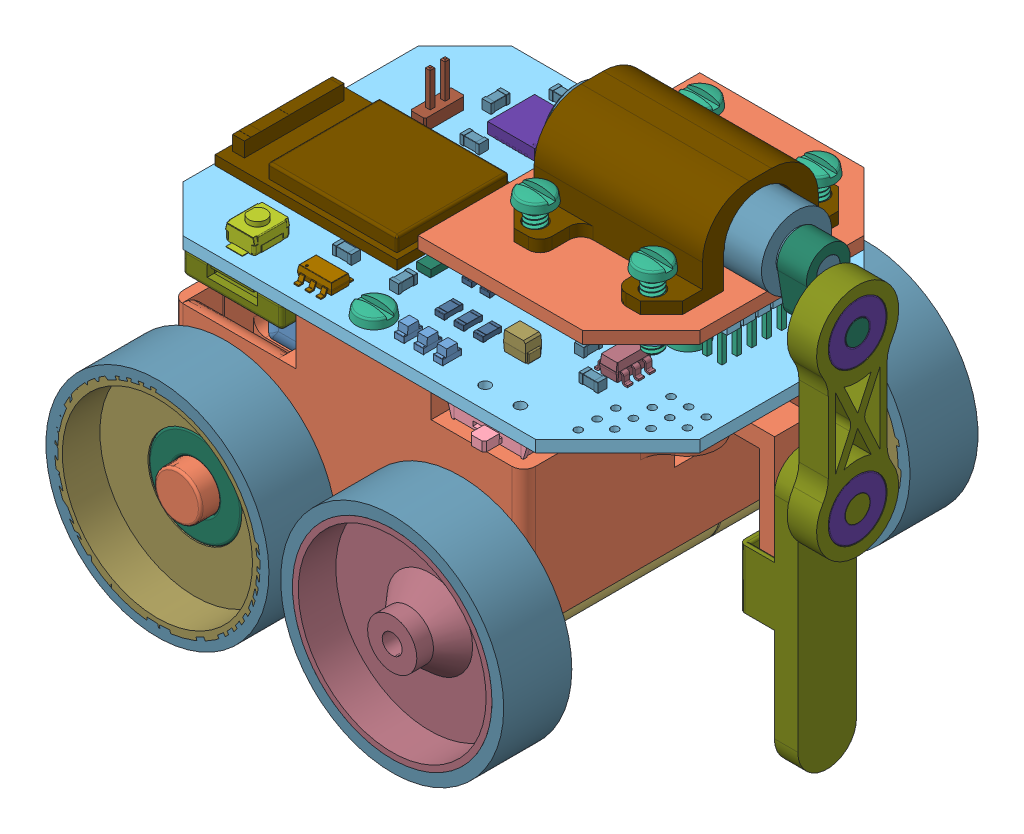
SolidWorks assembly AstroAnt_knock, configuration Default. Lengths in mm.
Overall size (52.98 43.52 40.4).
186 component instances, 53 part files, 54 mates.
Components (placement in the parent):
- LiPo_360mAh-1: LiPo_360mAh [Default] at (6.8166 4.9998 44.2756) size (25 7 18)
- Body-1: Body [Default] at (4.8007 -0.0002 38.7677) size (39 16 37)
- PA2-50-1: PA2-50 [Default] at (8.0673 -18.301 41.8029) x (0 0 1) z (0.952879 0.303349 0) size (29.1 8 8)
- PA2-50-2: PA2-50 [Default] at (-4.1563 19.5334 49.6029) x (0 0 -1) z (0.755989 -0.654584 0) size (29.1 8 8)
- 92120A150_Brass Heat-Set Inserts for Plastic-1: 92120A150_Brass Heat-Set Inserts for Plastic [92120A150] at (19.9543 12.4998 45.7029) size (2.56 3.33 2.56)
- 92120A150_Brass Heat-Set Inserts for Plastic-2: 92120A150_Brass Heat-Set Inserts for Plastic [92120A150] at (4.9543 12.4998 33.9529) size (2.56 3.33 2.56)
- 92120A150_Brass Heat-Set Inserts for Plastic-3: 92120A150_Brass Heat-Set Inserts for Plastic [92120A150] at (4.9543 12.4998 57.4529) size (2.56 3.33 2.56)
- motor_holder-1: motor_holder [Default] at (-0.192 -4.5002 11.9282) size (20 4.13 28)
- 91460A005_METRIC CHEESE HEAD SLOTTED MACHINE SCREW-8: 91460A005_METRIC CHEESE HEAD SLOTTED MACHINE SCREW [91460A005] at (4.9543 14.9998 57.4529) x (1 0 0) z (0 1 0) size (3 3 7.1)
- 91460A005_METRIC CHEESE HEAD SLOTTED MACHINE SCREW-9: 91460A005_METRIC CHEESE HEAD SLOTTED MACHINE SCREW [91460A005] at (4.9543 14.9998 33.9529) x (1 0 0) z (0 1 0) size (3 3 7.1)
- 91460A005_METRIC CHEESE HEAD SLOTTED MACHINE SCREW-10: 91460A005_METRIC CHEESE HEAD SLOTTED MACHINE SCREW [91460A005] at (19.9543 14.9998 45.7029) x (1 0 0) z (0 1 0) size (3 3 7.1)
- 92120A150_Brass Heat-Set Inserts for Plastic-4: 92120A150_Brass Heat-Set Inserts for Plastic [92120A150] at (4.9543 1.4998 57.4529) x (-0.616962 0 -0.786993) z (0.786993 0 -0.616962) size (2.56 3.33 2.56)
- 92120A150_Brass Heat-Set Inserts for Plastic-5: 92120A150_Brass Heat-Set Inserts for Plastic [92120A150] at (4.9543 1.4998 33.9529) x (-0.616962 0 -0.786993) z (0.786993 0 -0.616962) size (2.56 3.33 2.56)
- 91460A005_METRIC CHEESE HEAD SLOTTED MACHINE SCREW-14: 91460A005_METRIC CHEESE HEAD SLOTTED MACHINE SCREW [91460A005] at (4.9543 -2.5002 57.4529) x (0.663599 0 0.748089) z (0 -1 0) size (3 3 7.1)
- 91460A005_METRIC CHEESE HEAD SLOTTED MACHINE SCREW-15: 91460A005_METRIC CHEESE HEAD SLOTTED MACHINE SCREW [91460A005] at (4.9543 -2.5002 33.9529) x (0.663599 0 0.748089) z (0 -1 0) size (3 3 7.1)
- mainboard_v1.step-1: mainboard_v1.step [Default] at (-103.0457 13.9998 235.7029) x (0 0 -1) z (0 1 0) size (29.41 41 10.8)
  - B3U-1000P.step-1: B3U-1000P.step [Default] at (178.95 -97.38 1.05) x (1 0 0) z (0 -1 0) size (4 1.75 2.5)
    - COMPOUND.step-1: COMPOUND.step [Default] at origin size (4 1.75 2.5)
  - 20021321-00014C1LF.step-1: 20021321-00014C1LF.step [Default] at (190 -115.5 1.05) size (9.35 5.45 4.85)
    - COMPOUND-0.step-1: COMPOUND-0.step [Default] at origin size (9.35 5.45 4.85)
  - MP6513GJ-Z.step-1: MP6513GJ-Z.step [Default] at (201.21 -120 1.05) x (-1 0 0) z (0 0 1) size (2.8 2.9 1)
    - COMPOUND-1.step-1: COMPOUND-1.step [Default] at origin size (2.8 2.9 1)
  - MP6513GJ-Z.step-2: MP6513GJ-Z.step [Default] at (178.51 -103.46 1.05) size (2.8 2.9 1)
    - COMPOUND-1.step-1: COMPOUND-1.step [Default] at origin size (2.8 2.9 1)
  - R_0603_1608Metric.step-1: R_0603_1608Metric.step [Default] at (195.55 -104.38 -0.05) x (1 0 0) z (0 0 -1) size (1.6 0.8 0.45)
    - SOLID.step-1: SOLID.step [Default] at origin size (1.6 0.8 0.45)
  - R_0603_1608Metric.step-2: R_0603_1608Metric.step [Default] at (192.6 -99.86 -0.05) x (0 1 0) z (0 0 -1) size (1.6 0.8 0.45)
    - SOLID.step-1: SOLID.step [Default] at origin size (1.6 0.8 0.45)
  - PinHeader_2x01_P1.27mm_Vertical.step-1: PinHeader_2x01_P1.27mm_Vertical.step [Default] at (194.96 -96.07 1.05) size (3.4 1.27 6.3)
    - SOLID-2.step-1: SOLID-2.step [Default] at origin size (3.4 1.27 6.3)
  - TAJP106K010RNJ.step-1: TAJP106K010RNJ.step [Default] at (196.22 -98.14 -0.05) x (-1 0 0) z (0 0 -1) size (2.05 1.4 1.7)
    - COMPOUND-3.step-1: COMPOUND-3.step [Default] at origin size (2.05 1.4 1.7)
  - TAJP106K010RNJ.step-2: TAJP106K010RNJ.step [Default] at (181.68 -117.23 1.05) x (0 1 0) z (0 0 1) size (2.05 1.4 1.7)
    - COMPOUND-3.step-1: COMPOUND-3.step [Default] at origin size (2.05 1.4 1.7)
  - SOT-23-5.step-1: SOT-23-5.step [Default] at (195.38 -122.78 1.05) x (0 1 0) z (0 0 1) size (2.8 2.9 1.55)
    - SOLID-4.step-1: SOLID-4.step [Default] at origin size (2.8 2.9 1.55)
  - C_0603_1608Metric.step-1: C_0603_1608Metric.step [Default] at (192.91 -122.55 1.05) x (0 -1 0) z (0 0 1) size (1.6 0.8 0.8)
    - SOLID-5.step-1: SOLID-5.step [Default] at origin size (1.6 0.8 0.8)
  - C_0603_1608Metric.step-2: C_0603_1608Metric.step [Default] at (193.57 -119.76 1.05) size (1.6 0.8 0.8)
    - SOLID-5.step-1: SOLID-5.step [Default] at origin size (1.6 0.8 0.8)
  - ECS-.327-12.5-12-TR.step-1: ECS-.327-12.5-12-TR.step [Default] at (184.31 -107.18 1.05) size (2 1.2 0.7)
    - COMPOUND-6.step-1: COMPOUND-6.step [Default] at origin size (2 1.2 0.7)
  - C_0603_1608Metric.step-3: C_0603_1608Metric.step [Default] at (197.67 -113.69 1.05) size (1.6 0.8 0.8)
    - SOLID-5.step-1: SOLID-5.step [Default] at origin size (1.6 0.8 0.8)
  - C_0603_1608Metric.step-4: C_0603_1608Metric.step [Default] at (197.64 -107.18 1.05) size (1.6 0.8 0.8)
    - SOLID-5.step-1: SOLID-5.step [Default] at origin size (1.6 0.8 0.8)
  - C_0603_1608Metric.step-5: C_0603_1608Metric.step [Default] at (190.96 -108.09 1.05) x (0 1 0) z (0 0 1) size (1.6 0.8 0.8)
    - SOLID-5.step-1: SOLID-5.step [Default] at origin size (1.6 0.8 0.8)
  - 1734592-6.step-1: 1734592-6.step [Default] at (203.79 -118 -1.05) x (0 -1 0) z (1 0 0) size (8.43 2.05 5.11)
    - SOLID-7.step-1: SOLID-7.step [Default] at origin size (8.43 2.05 5.11)
  - 1734592-6.step-2: 1734592-6.step [Default] at (176.19 -98 -1.05) x (0 1 0) z (-1 0 0) size (8.43 2.05 5.11)
    - SOLID-7.step-1: SOLID-7.step [Default] at origin size (8.43 2.05 5.11)
  - 20021321-00010C4LF.step-1: 20021321-00010C4LF.step [Default] at (190 -127.85 -0.05) x (1 0 0) z (0 0 -1) size (6.81 5.45 4.85)
    - COMPOUND-8.step-1: COMPOUND-8.step [Default] at origin size (6.81 5.45 4.85) (hidden)
  - 20021321-00010C4LF.step-2: 20021321-00010C4LF.step [Default] at (190 -127.85 1.05) size (6.81 5.45 4.85)
    - COMPOUND-8.step-1: COMPOUND-8.step [Default] at origin size (6.81 5.45 4.85) (hidden)
  - C_0603_1608Metric.step-6: C_0603_1608Metric.step [Default] at (181.31 -102.6 1.05) x (0 -1 0) z (0 0 1) size (1.6 0.8 0.8)
    - SOLID-5.step-1: SOLID-5.step [Default] at origin size (1.6 0.8 0.8)
  - C_0603_1608Metric.step-7: C_0603_1608Metric.step [Default] at (198.25 -119.14 1.05) x (0 -1 0) z (0 0 1) size (1.6 0.8 0.8)
    - SOLID-5.step-1: SOLID-5.step [Default] at origin size (1.6 0.8 0.8)
  - MPU6050.step-1: MPU6050.step [Default] at (198.43 -101.5 1.05) x (0 1 0) z (1 0 0) size (4 0.95 4)
    - COMPOUND-9.step-1: COMPOUND-9.step [Default] at origin size (4 0.95 4)
  - C_0603_1608Metric.step-8: C_0603_1608Metric.step [Default] at (194.9 -99.89 1.05) x (0 -1 0) z (0 0 1) size (1.6 0.8 0.8)
    - SOLID-5.step-1: SOLID-5.step [Default] at origin size (1.6 0.8 0.8)
  - C_0603_1608Metric.step-9: C_0603_1608Metric.step [Default] at (201.98 -100.38 1.05) x (0 -1 0) z (0 0 1) size (1.6 0.8 0.8)
    - SOLID-5.step-1: SOLID-5.step [Default] at origin size (1.6 0.8 0.8)
  - C_0603_1608Metric.step-10: C_0603_1608Metric.step [Default] at (201.98 -103.78 1.05) x (0 1 0) z (0 0 1) size (1.6 0.8 0.8)
    - SOLID-5.step-1: SOLID-5.step [Default] at origin size (1.6 0.8 0.8)
  - C_0603_1608Metric.step-11: C_0603_1608Metric.step [Default] at (198.81 -97.82 1.05) size (1.6 0.8 0.8)
    - SOLID-5.step-1: SOLID-5.step [Default] at origin size (1.6 0.8 0.8)
  - SOT-23-5.step-2: SOT-23-5.step [Default] at (184.86 -122.77 1.05) x (0 1 0) z (0 0 1) size (2.8 2.9 1.55)
    - SOLID-4.step-1: SOLID-4.step [Default] at origin size (2.8 2.9 1.55)
  - SOT-23-5.step-3: SOT-23-5.step [Default] at (197.58 -110.46 1.05) x (0 1 0) z (0 0 1) size (2.8 2.9 1.55)
    - SOLID-4.step-1: SOLID-4.step [Default] at origin size (2.8 2.9 1.55)
  - MDBT50Q-1MV2.step-1: MDBT50Q-1MV2.step [Default] at (187.3136 -98.605 1.0754) x (-1 0 0) z (0 1 0) size (10.5 2.06 15.5)
    - SOLID-10.step-1: SOLID-10.step [Default] at origin size (10.5 2.06 15.5)
  - C_0603_1608Metric.step-12: C_0603_1608Metric.step [Default] at (189.44 -108.09 1.05) x (0 1 0) z (0 0 1) size (1.6 0.8 0.8)
    - SOLID-5.step-1: SOLID-5.step [Default] at origin size (1.6 0.8 0.8)
  - C_0603_1608Metric.step-13: C_0603_1608Metric.step [Default] at (181.57 -107.18 1.05) x (-1 0 0) z (0 0 1) size (1.6 0.8 0.8)
    - SOLID-5.step-1: SOLID-5.step [Default] at origin size (1.6 0.8 0.8)
  - C_0603_1608Metric.step-14: C_0603_1608Metric.step [Default] at (186.97 -107.18 1.05) size (1.6 0.8 0.8)
    - SOLID-5.step-1: SOLID-5.step [Default] at origin size (1.6 0.8 0.8)
  - C_0603_1608Metric.step-15: C_0603_1608Metric.step [Default] at (184.77 -119.75 1.05) x (-1 0 0) z (0 0 1) size (1.6 0.8 0.8)
    - SOLID-5.step-1: SOLID-5.step [Default] at origin size (1.6 0.8 0.8)
  - C_0603_1608Metric.step-16: C_0603_1608Metric.step [Default] at (182.37 -122.54 1.05) x (0 -1 0) z (0 0 1) size (1.6 0.8 0.8)
    - SOLID-5.step-1: SOLID-5.step [Default] at origin size (1.6 0.8 0.8)
  - LED_0603_1608Metric.step-1: LED_0603_1608Metric.step [Default] at (178.19 -111.01 1.05) size (1.6 0.8 1.1)
    - SOLID-11.step-1: SOLID-11.step [Default] at origin size (1.6 0.8 1.1)
  - LED_0603_1608Metric.step-2: LED_0603_1608Metric.step [Default] at (178.19 -112.66 1.05) size (1.6 0.8 1.1)
    - SOLID-11.step-1: SOLID-11.step [Default] at origin size (1.6 0.8 1.1)
  - LED_0603_1608Metric.step-3: LED_0603_1608Metric.step [Default] at (178.19 -114.31 1.05) size (1.6 0.8 1.1)
    - SOLID-11.step-1: SOLID-11.step [Default] at origin size (1.6 0.8 1.1)
  - LED_0603_1608Metric.step-4: LED_0603_1608Metric.step [Default] at (202.34 -112.21 1.05) x (0 1 0) z (0 0 1) size (1.6 0.8 1.1)
    - SOLID-11.step-1: SOLID-11.step [Default] at origin size (1.6 0.8 1.1)
  - 473460001.step-1: 473460001.step [Default] at (201.68 -99.72 -1.25) x (0 -1 0) z (1 0 0) size (7.98 2.94 5.43)
    - COMPOUND-12.step-1: COMPOUND-12.step [Default] at origin size (7.98 2.94 5.43)
  - L_0603_1608Metric.step-1: L_0603_1608Metric.step [Default] at (192.48 -108.09 1.05) x (0 1 0) z (0 0 1) size (1.6 0.8 0.8)
    - SOLID-13.step-1: SOLID-13.step [Default] at origin size (1.6 0.8 0.8)
  - R_0603_1608Metric.step-3: R_0603_1608Metric.step [Default] at (185.18 -111.31 1.05) x (-1 0 0) z (0 0 1) size (1.6 0.8 0.45)
    - SOLID.step-1: SOLID.step [Default] at origin size (1.6 0.8 0.45)
  - R_0603_1608Metric.step-4: R_0603_1608Metric.step [Default] at (185.18 -109.77 1.05) size (1.6 0.8 0.45)
    - SOLID.step-1: SOLID.step [Default] at origin size (1.6 0.8 0.45)
  - R_0603_1608Metric.step-5: R_0603_1608Metric.step [Default] at (181.62 -111.01 1.05) size (1.6 0.8 0.45)
    - SOLID.step-1: SOLID.step [Default] at origin size (1.6 0.8 0.45)
  - R_0603_1608Metric.step-6: R_0603_1608Metric.step [Default] at (181.62 -112.66 1.05) size (1.6 0.8 0.45)
    - SOLID.step-1: SOLID.step [Default] at origin size (1.6 0.8 0.45)
  - R_0603_1608Metric.step-7: R_0603_1608Metric.step [Default] at (181.62 -114.31 1.05) x (-1 0 0) z (0 0 1) size (1.6 0.8 0.45)
    - SOLID.step-1: SOLID.step [Default] at origin size (1.6 0.8 0.45)
  - R_0603_1608Metric.step-8: R_0603_1608Metric.step [Default] at (194.84 -108.1 1.05) x (0 1 0) z (0 0 1) size (1.6 0.8 0.45)
    - SOLID.step-1: SOLID.step [Default] at origin size (1.6 0.8 0.45)
  - R_0603_1608Metric.step-9: R_0603_1608Metric.step [Default] at (200.69 -112.2325 1.05) x (0 1 0) z (0 0 1) size (1.6 0.8 0.45)
    - SOLID.step-1: SOLID.step [Default] at origin size (1.6 0.8 0.45)
  - R_0603_1608Metric.step-10: R_0603_1608Metric.step [Default] at (196.22 -101.51 -0.05) x (-1 0 0) z (0 0 -1) size (1.6 0.8 0.45)
    - SOLID.step-1: SOLID.step [Default] at origin size (1.6 0.8 0.45)
  - R_0603_1608Metric.step-11: R_0603_1608Metric.step [Default] at (196.22 -99.9725 -0.05) x (-1 0 0) z (0 0 -1) size (1.6 0.8 0.45)
    - SOLID.step-1: SOLID.step [Default] at origin size (1.6 0.8 0.45)
  - SW_SPDT_PCM12.step-1: SW_SPDT_PCM12.step [Default] at (178.18 -119.37 -0.05) x (0 1 0) z (0 0 -1) size (7.7 5 2)
    - SOLID-14.step-1: SOLID-14.step [Default] at origin size (7.7 5 2)
  - COMPOUND-15.step-1: COMPOUND-15.step [Default] at origin size (28 41 1)
- 91613A020_METRIC CHEESE HEAD SLOTTED MACHINE SCREW-1: 91613A020_METRIC CHEESE HEAD SLOTTED MACHINE SCREW [91613A020] at (1.2533 -0.5002 54.4029) x (1 0 0) z (0 1 0) size (3 3 5.08)
- 91613A020_METRIC CHEESE HEAD SLOTTED MACHINE SCREW-2: 91613A020_METRIC CHEESE HEAD SLOTTED MACHINE SCREW [91613A020] at (8.6533 -0.5002 54.4029) x (1 0 0) z (0 1 0) size (3 3 5.08)
- 91613A020_METRIC CHEESE HEAD SLOTTED MACHINE SCREW-3: 91613A020_METRIC CHEESE HEAD SLOTTED MACHINE SCREW [91613A020] at (1.2533 -0.5002 37.0029) x (1 0 0) z (0 1 0) size (3 3 5.08)
- IR_TEMP_V2.step-3: IR_TEMP_V2.step [Default] at (118.9553 -0.5002 109.7029) x (-1 0 0) z (0 1 0) size (10 20 4.8)
  - Board_Geoms_380f.step-1: Board_Geoms_380f.step [Default] at origin size (10 20 1.11)
    - Pcb_380f.step-1: Pcb_380f.step [Default] at origin size (10 20 1)
    - topTracks_380f.step-1: topTracks_380f.step [Default] at (0 0 0.01) size (9.62 17.53 0.05)
    - botTracks_380f.step-1: botTracks_380f.step [Default] at (0 0 -1.01) size (9.25 16.88 0.05)
  - Step_Models_380f.step-1: Step_Models_380f.step [Default] at origin size (9.46 10.17 4.8)
    - Top_380f.step-1: Top_380f.step [Default] at origin size (9.46 10.17 1.2)
      - IC1_PW14_613E6C6D.step-1: IC1_PW14_613E6C6D.step [Default] at (113.99 -59.48 0) x (-1 0 0) z (0 1 0) size (6.4 1.2 5)
      - C1_C_0402_1005Metric_613EDDF6.step-1: C1_C_0402_1005Metric_613EDDF6.step [Default] at (110.5 -64.26 0) x (-1 0 0) z (0 0 1) size (1 0.5 0.5)
      - C1_C_0402_1005Metric_613EDDF6.step-2: C1_C_0402_1005Metric_613EDDF6.step [Default] at (109.52 -61.07 0) x (0 -1 0) z (0 0 1) size (1 0.5 0.5)
      - C1_C_0402_1005Metric_613EDDF6.step-3: C1_C_0402_1005Metric_613EDDF6.step [Default] at (118.48 -60.86 0) x (0 -1 0) z (0 0 1) size (1 0.5 0.5)
      - C1_C_0402_1005Metric_613EDDF6.step-4: C1_C_0402_1005Metric_613EDDF6.step [Default] at (118.48 -58.59 0) x (0 -1 0) z (0 0 1) size (1 0.5 0.5)
      - C1_C_0402_1005Metric_613EDDF6.step-5: C1_C_0402_1005Metric_613EDDF6.step [Default] at (113.32 -66.9 0) size (1 0.5 0.5)
      - R1_R_0402_1005Metric_613EDE7A.step-1: R1_R_0402_1005Metric_613EDE7A.step [Default] at (110.98 -63.1 0) size (1 0.5 0.35)
      - R1_R_0402_1005Metric_613EDE7A.step-2: R1_R_0402_1005Metric_613EDE7A.step [Default] at (111.68 -66.3 0) x (0 1 0) z (0 0 1) size (1 0.5 0.35)
    - Bot_380f.step-1: Bot_380f.step [Default] at origin size (6.35 7.64 4.6)
      - U1_ZTP-135SR_613E6CD4.step-1: U1_ZTP-135SR_613E6CD4.step [Default] at (114 -64 -1) x (-1 0 0) z (0 -1 0) size (6.35 4.6 5.4)
      - C1_C_0402_1005Metric_613EDDF6.step-1: C1_C_0402_1005Metric_613EDDF6.step [Default] at (115.07 -59.56 -1) x (0 -1 0) z (0 0 -1) size (1 0.5 0.5)
      - R1_R_0402_1005Metric_613EDE7A.step-1: R1_R_0402_1005Metric_613EDE7A.step [Default] at (113.64 -59.58 -1) x (0 -1 0) z (0 0 -1) size (1 0.5 0.35)
- TGPP06-D-136-1: TGPP06-D-136 [Default] at (10.3043 25.9998 45.7013) x (0 0.096627 0.995321) z (1 0 0) size (6 6 21.6)
- knock_wheel-1: knock_wheel [Default] at (29.4043 58.5713 96.4623) x (1 0 0) z (0 -0.096627 -0.995321) size (5.3 6.04 3.72)
- knock_connect_bar-1: knock_connect_bar [Default] at (32.2043 -15.7821 12.5082) size (2.5 20 7)
- ball_bearing-1: ball_bearing [Default] at (32.2043 22.8882 46.0034) x (1 0 0) z (0 -0.605691 0.7957) size (2.5 5 5)
- ball_bearing-2: ball_bearing [Default] at (32.2043 9.8882 46.0034) size (2.5 5 5)
- knock_motor_holder-1: knock_motor_holder [Default] at (-0.3495 23.0998 0.3235) size (14.34 7 16.88)
- 91460A005_METRIC CHEESE HEAD SLOTTED MACHINE SCREW-16: 91460A005_METRIC CHEESE HEAD SLOTTED MACHINE SCREW [91460A005] at (23.9543 25.5998 38.7029) x (1 0 0) z (0 1 0) size (3 3 7.1)
- 91460A005_METRIC CHEESE HEAD SLOTTED MACHINE SCREW-17: 91460A005_METRIC CHEESE HEAD SLOTTED MACHINE SCREW [91460A005] at (13.9543 25.5998 38.7029) x (1 0 0) z (0 1 0) size (3 3 7.1)
- 91460A005_METRIC CHEESE HEAD SLOTTED MACHINE SCREW-18: 91460A005_METRIC CHEESE HEAD SLOTTED MACHINE SCREW [91460A005] at (23.9543 25.5998 52.7013) x (1 0 0) z (0 1 0) size (3 3 7.1)
- 91460A005_METRIC CHEESE HEAD SLOTTED MACHINE SCREW-19: 91460A005_METRIC CHEESE HEAD SLOTTED MACHINE SCREW [91460A005] at (13.9543 25.5998 52.7013) x (1 0 0) z (0 1 0) size (3 3 7.1)
- 90710A145_18-8 Stainless Steel Thin Hex Nut-1: 90710A145_18-8 Stainless Steel Thin Hex Nut [90710A145] at (23.9543 21.4998 52.7029) size (3.2 1.33 3.7)
- 90710A145_18-8 Stainless Steel Thin Hex Nut-2: 90710A145_18-8 Stainless Steel Thin Hex Nut [90710A145] at (23.9543 21.4998 38.7029) size (3.2 1.33 3.7)
- 90710A145_18-8 Stainless Steel Thin Hex Nut-3: 90710A145_18-8 Stainless Steel Thin Hex Nut [90710A145] at (13.9543 21.4998 38.7029) size (3.2 1.33 3.7)
- 90710A145_18-8 Stainless Steel Thin Hex Nut-4: 90710A145_18-8 Stainless Steel Thin Hex Nut [90710A145] at (13.9543 21.4998 52.7029) size (3.2 1.33 3.7)
- knock_driver.step-1: knock_driver.step [Default] at (27.9543 23.0401 52.7029) x (0 0 -1) z (0 1 0) size (24 19 6.04)
  - Board.step-1: Board.step [Default] at origin size (24 19 1.04)
    - Open CASCADE STEP translator 6.8 3.1.1.step-1: Open CASCADE STEP translator 6.8 3.1.1.step [Default] at (0 0 -1.0403) size (24 19 1.04)
  - J4.step-1: J4.step [Default] at origin size (6.35 5.1 5)
    - 5183718160.step-1: 5183718160.step [Default] at (7 15.55 -1.0403) x (-1 0 0) z (0 0 -1) size (6.35 5.1 5)
      - Body.step-1: Body.step [Default] at origin size (6.35 3.4 1)
      - LeadsArray.step-1: LeadsArray.step [Default] at origin size (5.48 5.1 5)
  - J3.step-1: J3.step [Default] at origin size (6.35 5.1 5)
    - 5181933872.step-1: 5181933872.step [Default] at (7 3.2 -1.0403) x (1 0 0) z (0 0 -1) size (6.35 5.1 5)
      - Body-0.step-1: Body-0.step [Default] at origin size (6.35 3.4 1)
      - LeadsArray-1.step-1: LeadsArray-1.step [Default] at origin size (5.48 5.1 5)
  - IC1.step-1: IC1.step [Default] at origin size (2.9 2.8 1)
    - 7744092656.step-1: 7744092656.step [Default] at (7 9.2972 -1.0403) x (0 1 0) z (0 0 -1) size (2.8 2.9 1)
      - Body-2.step-1: Body-2.step [Default] at origin size (1.6 2.9 0.95)
      - PinsArrayLR.step-1: PinsArrayLR.step [Default] at origin size (2.8 2.3 0.54)
  - C1.step-1: C1.step [Default] at origin size (1.6 0.8 0.9)
    - Cap_Murata_GCM1885C2A5R3BA16J_eec.step-1: Cap_Murata_GCM1885C2A5R3BA16J_eec.step [Default] at (3.3028 10.1862 -1.0403) x (-1 0 0) z (0 0 -1) size (1.6 0.8 0.9)
      - 1.step-1: 1.step [Default] at origin size (1.6 0.8 0.9)
      - 2.step-1: 2.step [Default] at origin size (0.9 0.8 0.9)
      - Murata_Logo_3.step-1: Murata_Logo_3.step [Default] at (-0.526 -1.4102 0.801) size (0.36 0.08 0.1)
- wheel_holder_non_motor-1: wheel_holder_non_motor [Default] at (-70.2522 1.7638 25.5029) size (17.5 17.5 5.8)
- wheel_motor-1: wheel_motor [Default] at (24.0366 1.7037 25.5029) size (17 17 5.8)
- tire-1: tire [Default] at (-28.6116 -36.2502 65.9029) x (-0.5727 -0.819765 0) z (0 0 -1) size (19 19 5.8)
- tire-2: tire [Default] at (-13.1847 -32.8271 65.9029) x (-0.675771 -0.737112 0) z (0 0 -1) size (19 19 5.8)
- tire-3: tire [Default] at (58.167 -1.442 25.5029) size (19 19 5.8)
- tire-4: tire [Default] at (38.167 -1.442 25.5029) size (19 19 5.8)
- wheel_motor-2: wheel_motor [Default] at (-11.7392 -11.668 65.9029) x (-0.891298 -0.453419 0) z (0 0 -1) size (17 17 5.8)
- wheel_holder_non_motor-2: wheel_holder_non_motor [Default] at (44.8061 -69.1237 65.9029) x (-0.568031 0.823007 0) z (0 0 -1) size (17.5 17.5 5.8)
- ball_bearing_5x11x4mm-1: ball_bearing_5x11x4mm [Default] at (-65.4312 -2.9154 60.2029) size (8 8 2.5)
- ball_bearing_5x11x4mm-2: ball_bearing_5x11x4mm [Default] at (-45.4312 -2.9154 28.7029) size (8 8 2.5)
- knock_knob-2: knock_knob [Default] at (30.1043 -5.6273 31.2685) size (7.6 23 5)
Mates (geometry in assembly coordinates):
- Coincident51: coincident anti-aligned: plane of LiPo_360mAh-1 through (6.8166 4.9998 44.2756) normal (0 -1 0); plane of Body-1 through (4.8007 4.9998 38.7677) normal (0 1 0)
- Distance5: distance = 0.5 mm anti-aligned: plane of LiPo_360mAh-1 through (15.061 11.9998 36.7029) normal (0 0 -1); plane of Body-1 through (18.9543 4.9998 36.2029) normal (0 0 1)
- Coincident53: coincident aligned: plane of Body-1 through (4.8007 13.9998 38.7677) normal (0 1 0); plane of 92120A150_Brass Heat-Set Inserts for Plastic-1 through (18.8793 13.9998 45.7029) normal (0 1 0)
- Concentric38: concentric aligned: cylinder of Body-1 through (19.9543 5.9998 45.7029) axis (0 1 0) radius 1.15; cylinder of 92120A150_Brass Heat-Set Inserts for Plastic-1 through (19.9543 13.9998 45.7029) axis (0 1 0) radius 1.075
- Coincident55: coincident aligned: plane of Body-1 through (4.8007 13.9998 38.7677) normal (0 1 0); plane of 92120A150_Brass Heat-Set Inserts for Plastic-3 through (3.8793 13.9998 57.4529) normal (0 1 0)
- Concentric39: concentric aligned: cylinder of Body-1 through (4.9543 -2.0002 57.4529) axis (0 1 0) radius 1.15; cylinder of 92120A150_Brass Heat-Set Inserts for Plastic-3 through (4.9543 13.9998 57.4529) axis (0 1 0) radius 1.075
- Coincident56: coincident aligned: plane of Body-1 through (4.8007 13.9998 38.7677) normal (0 1 0); plane of 92120A150_Brass Heat-Set Inserts for Plastic-2 through (3.8793 13.9998 33.9529) normal (0 1 0)
- Concentric40: concentric aligned: cylinder of Body-1 through (4.9543 -2.0002 33.9529) axis (0 1 0) radius 1.15; cylinder of 92120A150_Brass Heat-Set Inserts for Plastic-2 through (4.9543 13.9998 33.9529) axis (0 1 0) radius 1.075
- Coincident57: coincident anti-aligned: plane of LiPo_360mAh-1 through (6.8166 4.9998 44.2756) normal (0 -1 0); plane of Body-1 through (4.8007 4.9998 38.7677) normal (0 1 0)
- Coincident70: coincident aligned: plane of Body-1 through (-10.0457 13.9998 31.7029) normal (0 0 -1); plane of motor_holder-1 through (14.9553 -0.5002 31.7029) normal (0 0 -1)
- Concentric47: concentric aligned: cylinder of Body-1 through (4.9543 -2.0002 57.4529) axis (0 1 0) radius 1.15; cylinder of 92120A150_Brass Heat-Set Inserts for Plastic-4 through (4.9543 2.9998 57.4529) axis (0 1 0) radius 1.075
- Concentric48: concentric aligned: cylinder of Body-1 through (4.9543 -2.0002 33.9529) axis (0 1 0) radius 1.15; cylinder of 92120A150_Brass Heat-Set Inserts for Plastic-5 through (4.9543 2.9998 33.9529) axis (0 1 0) radius 1.075
- Coincident89: coincident aligned: plane of Body-1 through (4.8007 -0.0002 38.7677) normal (0 -1 0); plane of 92120A150_Brass Heat-Set Inserts for Plastic-5 through (5.4479 -0.0002 34.5825) normal (0 -1 0)
- Coincident90: coincident aligned: plane of Body-1 through (4.8007 -0.0002 38.7677) normal (0 -1 0); plane of 92120A150_Brass Heat-Set Inserts for Plastic-4 through (5.4479 -0.0002 58.0825) normal (0 -1 0)
- Concentric59: concentric aligned: circle of TGPP06-D-136-1; circle of knock_wheel-1
- Coincident104: coincident anti-aligned: plane of TGPP06-D-136-1 through (29.4043 25.9998 45.7013) normal (1 0 0); plane of knock_wheel-1 through (29.4043 22.8882 46.0034) normal (-1 0 0)
- Concentric60: concentric anti-aligned: circle of knock_wheel-1; circle of ball_bearing-1
- Coincident105: coincident aligned: plane of knock_wheel-1 through (34.7043 22.8882 46.0034) normal (1 0 0); plane of ball_bearing-1 through (34.7043 22.8882 46.0034) normal (1 0 0)
- Concentric62: concentric anti-aligned: cylinder of knock_connect_bar-1 through (32.2043 22.8882 46.0034) axis (1 0 0) radius 2.51; cylinder of ball_bearing-1 through (34.7043 22.8882 46.0034) axis (-1 0 0) radius 2.5
- Coincident106: coincident aligned: plane of knock_connect_bar-1 through (34.7043 22.8882 46.0034) normal (1 0 0); plane of ball_bearing-1 through (34.7043 22.8882 46.0034) normal (1 0 0)
- Coincident107: coincident aligned: plane of knock_connect_bar-1 through (34.7043 22.8882 46.0034) normal (1 0 0); plane of ball_bearing-2 through (34.7043 9.8882 46.0034) normal (1 0 0)
- Concentric63: concentric anti-aligned: cylinder of knock_connect_bar-1 through (32.2043 9.8882 46.0034) axis (1 0 0) radius 2.51; cylinder of ball_bearing-2 through (34.7043 9.8882 46.0034) axis (-1 0 0) radius 2.5
- Concentric69: concentric aligned: cylinder of TGPP06-D-136-1 through (19.2043 25.9998 45.7013) axis (-1 0 0) radius 3; cylinder of knock_motor_holder-1 through (26.1243 25.9998 45.7013) axis (-1 0 0) radius 3.1
- Parallel3: parallel anti-aligned: plane of TGPP06-D-136-1 through (31.9043 25.5121 45.7486) normal (0 -0.995321 0.096627); plane of knock_wheel-1 through (27.2373 25.4037 44.7578) normal (0 0.995321 -0.096627)
- Coincident126: coincident aligned: plane of mainboard_v1.step-1/COMPOUND-15.step-1 through (27.9543 13.9998 38.7029) normal (1 0 0); plane of knock_driver.step-1/Board.step-1/Open CASCADE STEP translator 6.8 3.1.1.step-1 through (27.9543 21.9998 52.7029) normal (1 0 0)
- Coincident127: coincident anti-aligned: plane of 90710A145_18-8 Stainless Steel Thin Hex Nut-3 through (12.3543 21.9998 37.7791) normal (0 1 0); plane of knock_driver.step-1/Board.step-1/Open CASCADE STEP translator 6.8 3.1.1.step-1 through (22.9543 21.9998 57.7029) normal (0 -1 0)
- Coincident128: coincident aligned: plane of mainboard_v1.step-1/COMPOUND-15.step-1 through (20.9543 13.9998 31.7029) normal (0.707107 0 -0.707107); plane of knock_driver.step-1/Board.step-1/Open CASCADE STEP translator 6.8 3.1.1.step-1 through (27.9543 21.9998 38.7029) normal (0.707107 0 -0.707107)
- Concentric77: concentric anti-aligned: cylinder of motor_holder-1 through (4.9543 -2.5002 57.4529) axis (0 -1 0) radius 1.75; circle of 91460A005_METRIC CHEESE HEAD SLOTTED MACHINE SCREW-14
- Concentric79: concentric anti-aligned: cylinder of PA2-50-1 through (14.9543 -0.0002 58.0029) axis (0 0 -1) radius 4; cylinder of motor_holder-1 through (14.9543 -0.0002 34.2029) axis (0 0 1) radius 4.05
- Concentric80: concentric anti-aligned: cylinder of wheel_motor-1 through (-5.0457 -0.0002 31.3029) axis (0 0 -1) radius 8.5; cylinder of tire-4 through (-5.0457 -0.0002 25.5029) axis (0 0 1) radius 8.5
- Coincident129: coincident aligned: plane of wheel_motor-1 through (-5.0457 -0.0002 25.5029) normal (0 0 -1); plane of tire-4 through (-5.0457 -0.0002 25.5029) normal (0 0 -1)
- Concentric81: concentric anti-aligned: cylinder of wheel_holder_non_motor-1 through (14.9543 -0.0002 31.3029) axis (0 0 -1) radius 8.75; cylinder of tire-3 through (14.9543 -0.0002 25.5029) axis (0 0 1) radius 8.5
- Coincident130: coincident aligned: plane of wheel_holder_non_motor-1 through (14.9543 -0.0002 25.5029) normal (0 0 -1); plane of tire-3 through (14.9543 -0.0002 25.5029) normal (0 0 -1)
- Concentric82: concentric anti-aligned: cylinder of tire-2 through (14.9543 -0.0002 65.9029) axis (0 0 -1) radius 8.5; cylinder of wheel_motor-2 through (14.9543 -0.0002 60.1029) axis (0 0 1) radius 8.5
- Concentric83: concentric anti-aligned: cylinder of tire-1 through (-5.0457 -0.0002 65.9029) axis (0 0 -1) radius 8.5; cylinder of wheel_holder_non_motor-2 through (-5.0457 -0.0002 60.1029) axis (0 0 1) radius 8.75
- Coincident131: coincident aligned: plane of tire-1 through (-5.0457 -0.0002 65.9029) normal (0 0 1); plane of wheel_holder_non_motor-2 through (-5.0457 -0.0002 65.9029) normal (0 0 1)
- Coincident132: coincident aligned: plane of tire-2 through (14.9543 -0.0002 65.9029) normal (0 0 1); plane of wheel_motor-2 through (14.9543 -0.0002 65.9029) normal (0 0 1)
- Concentric84: concentric anti-aligned: cylinder of PA2-50-2 through (-5.0457 -0.0002 28.3029) axis (0 0 1) radius 0.5; cylinder of wheel_motor-1 through (-5.0457 -0.0002 31.3029) axis (0 0 -1) radius 0.85
- Coincident133: coincident anti-aligned: plane of PA2-50-2 through (-5.0457 -0.0002 31.3029) normal (0 0 -1); plane of wheel_motor-1 through (-5.0457 -0.0002 31.3029) normal (0 0 1)
- Concentric85: concentric aligned: cylinder of Body-1 through (14.9543 -0.0002 27.2029) axis (0 0 1) radius 2; cylinder of wheel_holder_non_motor-1 through (14.9543 -0.0002 25.5029) axis (0 0 1) radius 4
- Concentric86: concentric aligned: cylinder of PA2-50-1 through (14.9543 -0.0002 62.1029) axis (0 0 -1) radius 1; cylinder of wheel_motor-2 through (14.9543 -0.0002 63.1029) axis (0 0 -1) radius 1.1
- Coincident134: coincident anti-aligned: plane of PA2-50-1 through (14.9543 -0.0002 60.1029) normal (0 0 1); plane of wheel_motor-2 through (14.9543 -0.0002 60.1029) normal (0 0 -1)
- Concentric87: concentric aligned: cylinder of Body-1 through (-5.0457 -0.0002 64.2029) axis (0 0 -1) radius 2; cylinder of ball_bearing_5x11x4mm-1 through (-5.0457 -0.0002 64.2029) axis (0 0 -1) radius 2
- Coincident135: coincident aligned: plane of wheel_holder_non_motor-1 through (14.9543 -0.0002 28.7029) normal (0 0 -1); plane of ball_bearing_5x11x4mm-2 through (14.9543 -0.0002 28.7029) normal (0 0 -1)
- Concentric89: concentric anti-aligned: cylinder of wheel_holder_non_motor-1 through (14.9543 -0.0002 25.5029) axis (0 0 1) radius 4; cylinder of ball_bearing_5x11x4mm-2 through (14.9543 -0.0002 32.7029) axis (0 0 -1) radius 2
- Coincident136: coincident aligned: plane of tire-3 through (14.9543 -0.0002 25.5029) normal (0 0 -1); plane of tire-4 through (-5.0457 -0.0002 25.5029) normal (0 0 -1)
- Concentric90: concentric aligned: cylinder of wheel_holder_non_motor-2 through (-5.0457 -0.0002 65.9029) axis (0 0 -1) radius 4; cylinder of ball_bearing_5x11x4mm-1 through (-5.0457 -0.0002 62.7029) axis (0 0 -1) radius 4
- Coincident137: coincident aligned: plane of wheel_holder_non_motor-2 through (-5.0457 -0.0002 62.7029) normal (0 0 1); plane of ball_bearing_5x11x4mm-1 through (-5.0457 -0.0002 62.7029) normal (0 0 1)
- Coincident138: coincident aligned: plane of tire-1 through (-5.0457 -0.0002 65.9029) normal (0 0 1); plane of tire-2 through (14.9543 -0.0002 65.9029) normal (0 0 1)
- Concentric95: concentric aligned: cylinder of ball_bearing-2 through (34.7043 9.8882 46.0034) axis (-1 0 0) radius 1; cylinder of knock_knob-2 through (34.7043 9.8882 46.0034) axis (-1 0 0) radius 1.05
- Coincident143: coincident aligned: plane of knock_connect_bar-1 through (34.7043 22.8882 46.0034) normal (1 0 0); plane of knock_knob-2 through (34.7043 9.8882 46.0034) normal (1 0 0)
- Distance6: distance = 0.05 mm anti-aligned: plane of Body-1 through (27.6543 -0.5002 47.3324) normal (-1 0 0); plane of knock_knob-2 through (27.6043 -10.6118 48.0034) normal (1 0 0)
- Distance7: distance = 0.07 mm anti-aligned: plane of Body-1 through (28.9543 11.4998 44.0734) normal (0 0 -1); plane of knock_knob-2 through (29.6043 -10.6118 44.0034) normal (0 0 1)
- Parallel4: parallel aligned: plane of knock_connect_bar-1 through (34.7043 22.8882 48.5034) normal (0 0 1); plane of knock_driver.step-1/Board.step-1/Open CASCADE STEP translator 6.8 3.1.1.step-1 through (8.9543 21.9998 57.7029) normal (0 0 1)
